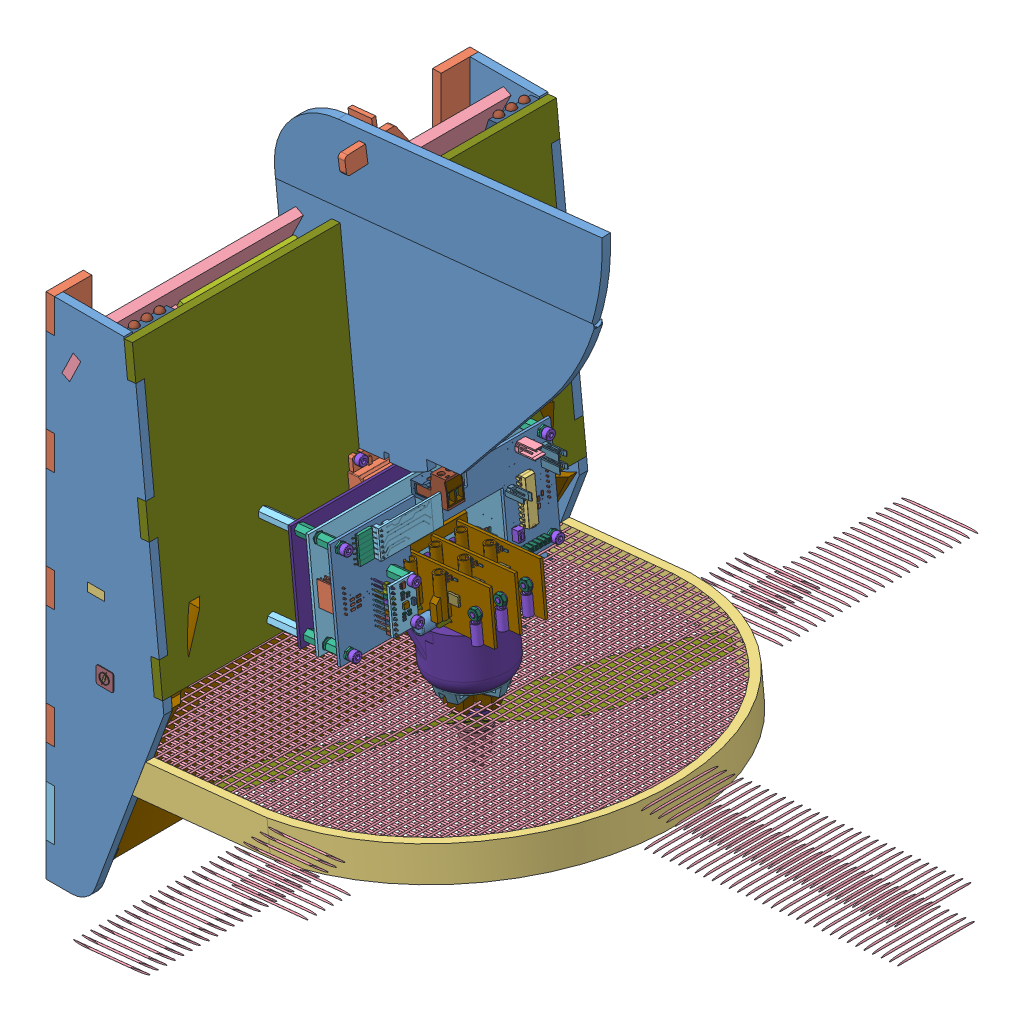
SolidWorks assembly AssTotale, configuration Défaut. Lengths in mm. (continued)
Components (placement in the parent): (continued)
- AssStructSimu-1: AssStructSimu [Défaut] at (-75.9431 -10.8604 24.5323) size (253.25 324.59 251.6) (continued)
  - AssCarte-1: AssCarte [Défaut] at (-42.8534 32.2132 302.028) x (-0.101852 0.9948 0) z (0.9948 0.101852 0) size (67.15 130.57 98.45) (continued)
    - carte_onduleur_v4-1: carte_onduleur_v4 [Défaut] at (-25.7639 0.8332 112.9379) size (66.52 130.57 82.34) (continued)
      - CARTE_ALIM-1: CARTE_ALIM [Défaut] at (-6.4 -57.2 0.803) size (60 130 18.35) (continued)
        - Open CASCADE STEP translator 6.8 1.63.1-1: Open CASCADE STEP translator 6.8 1.63.1 [Défaut] at origin size (60 130 18.35) (continued)
          - Body_1_6-1: Body_1_6 [Défaut] at (7 56 -12) size (60 130 18.35) (continued)
            - 109-1: 109 [Défaut] at (25.4933 -41.1272 0.803) x (-1 0 0) z (0 0 1) size (2.34 1.04 0.5) (continued)
              - =_[0_1_1_45]-1: =_[0_1_1_45] [Défaut] at origin size (2.34 1.04 0.5) (continued)
                - 51-1: 51 [Défaut] at origin size (0.51 1.02 0.5)
            - 111-1: 111 [Défaut] at (22.0269 -41.8272 0.803) x (-1 0 0) z (0 0 1) size (2.34 1.04 0.5)
              - =_[0_1_1_45]-1: =_[0_1_1_45] [Défaut] at origin size (2.34 1.04 0.5)
                - 49_3-1: 49_3 [Défaut] at origin size (2.29 1.04 0.43)
                - 50-1: 50 [Défaut] at (0.3048 0 0) x (-1 0 0) z (0 0 1) size (0.51 1.02 0.5)
                - 51-1: 51 [Défaut] at origin size (0.51 1.02 0.5)
            - 113-1: 113 [Défaut] at (-24.8 -36.7036 0.803) x (0 1 0) z (0 0 1) size (2.34 1.04 0.5)
              - =_[0_1_1_45]-1: =_[0_1_1_45] [Défaut] at origin size (2.34 1.04 0.5)
                - 49_3-1: 49_3 [Défaut] at origin size (2.29 1.04 0.43)
                - 50-1: 50 [Défaut] at (0.3048 0 0) x (-1 0 0) z (0 0 1) size (0.51 1.02 0.5)
                - 51-1: 51 [Défaut] at origin size (0.51 1.02 0.5)
            - 115-1: 115 [Défaut] at (-24.8 -40.3036 0.803) x (0 1 0) z (0 0 1) size (2.34 1.04 0.5)
              - =_[0_1_1_45]-1: =_[0_1_1_45] [Défaut] at origin size (2.34 1.04 0.5)
                - 49_3-1: 49_3 [Défaut] at origin size (2.29 1.04 0.43)
                - 50-1: 50 [Défaut] at (0.3048 0 0) x (-1 0 0) z (0 0 1) size (0.51 1.02 0.5)
                - 51-1: 51 [Défaut] at origin size (0.51 1.02 0.5)
            - 117-1: 117 [Défaut] at (-16 -48.27 0.803) x (0 -1 0) z (0 0 1) size (2.34 1.04 0.5)
              - =_[0_1_1_45]-1: =_[0_1_1_45] [Défaut] at origin size (2.34 1.04 0.5)
                - 49_3-1: 49_3 [Défaut] at origin size (2.29 1.04 0.43)
                - 50-1: 50 [Défaut] at (0.3048 0 0) x (-1 0 0) z (0 0 1) size (0.51 1.02 0.5)
                - 51-1: 51 [Défaut] at origin size (0.51 1.02 0.5)
            - 119-1: 119 [Défaut] at (-22.5189 -47.87 0.803) x (-1 0 0) z (0 0 1) size (2.34 1.04 0.5)
              - =_[0_1_1_45]-1: =_[0_1_1_45] [Défaut] at origin size (2.34 1.04 0.5)
                - 49_3-1: 49_3 [Défaut] at origin size (2.29 1.04 0.43)
                - 50-1: 50 [Défaut] at (0.3048 0 0) x (-1 0 0) z (0 0 1) size (0.51 1.02 0.5)
                - 51-1: 51 [Défaut] at origin size (0.51 1.02 0.5)
            - 121-1: 121 [Défaut] at (22.3933 -38.9272 0.803) size (2.34 1.04 0.5)
              - =_[0_1_1_45]-1: =_[0_1_1_45] [Défaut] at origin size (2.34 1.04 0.5)
                - 49_3-1: 49_3 [Défaut] at origin size (2.29 1.04 0.43)
                - 50-1: 50 [Défaut] at (0.3048 0 0) x (-1 0 0) z (0 0 1) size (0.51 1.02 0.5)
                - 51-1: 51 [Défaut] at origin size (0.51 1.02 0.5)
            - 123-1: 123 [Défaut] at (22.0933 -36.4272 0.803) x (-1 0 0) z (0 0 1) size (2.34 1.04 0.5)
              - =_[0_1_1_45]-1: =_[0_1_1_45] [Défaut] at origin size (2.34 1.04 0.5)
                - 49_3-1: 49_3 [Défaut] at origin size (2.29 1.04 0.43)
                - 50-1: 50 [Défaut] at (0.3048 0 0) x (-1 0 0) z (0 0 1) size (0.51 1.02 0.5)
                - 51-1: 51 [Défaut] at origin size (0.51 1.02 0.5)
            - 125-1: 125 [Défaut] at (22.3933 -32.0272 0.803) x (0 -1 0) z (0 0 1) size (2.34 1.04 0.5)
              - =_[0_1_1_45]-1: =_[0_1_1_45] [Défaut] at origin size (2.34 1.04 0.5)
                - 49_3-1: 49_3 [Défaut] at origin size (2.29 1.04 0.43)
                - 50-1: 50 [Défaut] at (0.3048 0 0) x (-1 0 0) z (0 0 1) size (0.51 1.02 0.5)
                - 51-1: 51 [Défaut] at origin size (0.51 1.02 0.5)
            - 127-1: 127 [Défaut] at (17.9597 -23.1272 0.803) size (2.34 1.04 0.5)
              - =_[0_1_1_16]-1: =_[0_1_1_16] [Défaut] at origin size (2.34 1.04 0.5)
                - 14_2-1: 14_2 [Défaut] at origin size (2.29 1.04 0.43)
                - 15_2-1: 15_2 [Défaut] at (0.3048 0 0) x (-1 0 0) z (0 0 1) size (0.51 1.02 0.5)
                - 16_2-1: 16_2 [Défaut] at origin size (0.51 1.02 0.5)
            - 129-1: 129 [Défaut] at (20.0269 -24.9272 0.803) x (-1 0 0) z (0 0 1) size (2.34 1.04 0.5)
              - =_[0_1_1_16]-1: =_[0_1_1_16] [Défaut] at origin size (2.34 1.04 0.5)
                - 14_2-1: 14_2 [Défaut] at origin size (2.29 1.04 0.43)
                - 15_2-1: 15_2 [Défaut] at (0.3048 0 0) x (-1 0 0) z (0 0 1) size (0.51 1.02 0.5)
                - 16_2-1: 16_2 [Défaut] at origin size (0.51 1.02 0.5)
            - 131-1: 131 [Défaut] at (16.9933 -37.5272 0.803) x (-1 0 0) z (0 0 1) size (2.34 1.04 0.5)
              - =_[0_1_1_45]-1: =_[0_1_1_45] [Défaut] at origin size (2.34 1.04 0.5)
                - 49_3-1: 49_3 [Défaut] at origin size (2.29 1.04 0.43)
                - 50-1: 50 [Défaut] at (0.3048 0 0) x (-1 0 0) z (0 0 1) size (0.51 1.02 0.5)
                - 51-1: 51 [Défaut] at origin size (0.51 1.02 0.5)
            - 136-1: 136 [Défaut] at (3.2957 -29.23 0.803) x (-1 0 0) z (0 0 1) size (4.78 2.79 2.03)
              - =_[0_1_1_110]_2-1: =_[0_1_1_110]_2 [Défaut] at origin size (4.78 2.79 2.03)
                - 132-1: 132 [Défaut] at origin size (4.32 2.79 1.78)
                - 133-1: 133 [Défaut] at (0.4572 0 0) x (-1 0 0) z (0 0 1) size (1.02 1.27 1.32)
                - 134-1: 134 [Défaut] at origin size (1.02 1.27 1.32)
            - 141-1: 141 [Défaut] at (0.2436 -33.3673 0.803) size (3.35 1.3 0.55)
              - =_[0_1_1_115]_2-1: =_[0_1_1_115]_2 [Défaut] at origin size (3.35 1.3 0.55)
                - 137-1: 137 [Défaut] at origin size (3.3 1.3 0.48)
                - 138-1: 138 [Défaut] at (0.5588 0 0) x (-1 0 0) z (0 0 1) size (0.76 1.27 0.55)
                - 139-1: 139 [Défaut] at origin size (0.76 1.27 0.55)
            - 143_2-1: 143_2 [Défaut] at (-0.3 -45.47 0.803) x (0 1 0) z (0 0 1) size (2.34 1.04 0.5)
              - =_[0_1_1_16]-1: =_[0_1_1_16] [Défaut] at origin size (2.34 1.04 0.5)
                - 14_2-1: 14_2 [Défaut] at origin size (2.29 1.04 0.43)
                - 15_2-1: 15_2 [Défaut] at (0.3048 0 0) x (-1 0 0) z (0 0 1) size (0.51 1.02 0.5)
                - 16_2-1: 16_2 [Défaut] at origin size (0.51 1.02 0.5)
            - 145-1: 145 [Défaut] at (6.6 31.13 0.803) x (0 1 0) z (0 0 1) size (3.35 1.3 0.55)
              - =_[0_1_1_25]_2-1: =_[0_1_1_25]_2 [Défaut] at origin size (3.35 1.3 0.55)
                - 24-1: 24 [Défaut] at origin size (3.3 1.3 0.48)
                - 25_2-1: 25_2 [Défaut] at (0.5588 0 0) x (-1 0 0) z (0 0 1) size (0.76 1.27 0.55)
                - 26_2-1: 26_2 [Défaut] at origin size (0.76 1.27 0.55)
            - 148-1: 148 [Défaut] at (-7.5 -56.57 0.803) size (15.24 2.54 7.37)
              - =_[0_1_1_122]_2-1: =_[0_1_1_122]_2 [Défaut] at origin size (15.24 2.54 7.37)
                - 146-1: 146 [Défaut] at (6.3 0 1) x (1 0 0) z (0 -1 0) size (15.24 7.37 2.54)
            - 150-1: 150 [Défaut] at (-26.3 -45.9 0.803) x (0 1 0) z (0 0 1) size (2.34 1.04 0.5)
              - =_[0_1_1_45]-1: =_[0_1_1_45] [Défaut] at origin size (2.34 1.04 0.5)
                - 49_3-1: 49_3 [Défaut] at origin size (2.29 1.04 0.43)
                - 50-1: 50 [Défaut] at (0.3048 0 0) x (-1 0 0) z (0 0 1) size (0.51 1.02 0.5)
                - 51-1: 51 [Défaut] at origin size (0.51 1.02 0.5)
    - AssEntretoise-1: AssEntretoise [Défaut] at (-50.7639 -62.5535 129.2811) x (0 0 -1) z (1 0 0) size (58.24 7.29 7.81)
      - socket head cap screw 4762_din-1: socket head cap screw 4762_din [EN ISO 4762 M3 x 5 - 5N] at (-2.4967 0.5867 0) size (8 5.5 5.5)
      - hexagonal_spacer_MF_M3_H20_HEX5.5_FTD6_MTL6-1: hexagonal_spacer_MF_M3_H20_HEX5.5_FTD6_MTL6 [Défaut] at (48.3433 0.5867 0) x (0 0 1) z (-1 0 0) size (6.36 5.51 26)
      - hex nut style 1 gradeab_din-1: hex nut style 1 gradeab_din [Hexagon Nut ISO 4032 - M3 - W - N] at (53.3433 0.5867 0) x (0 0.943962 0.330053) z (-1 0 0) size (5.5 6.35 2.4)
      - hexagonal_spacer_MF_M3_H12_HEX5.5_FTD6_MTL6-2: hexagonal_spacer_MF_M3_H12_HEX5.5_FTD6_MTL6 [Défaut] at (27.0633 0.5867 0) x (0 0.248308 0.968681) z (-1 0 0) size (6.36 5.51 18)
      - hexagonal_spacer_MF_M3_H12_HEX5.5_FTD6_MTL6-3: hexagonal_spacer_MF_M3_H12_HEX5.5_FTD6_MTL6 [Défaut] at (13.7833 0.5867 0) x (0 0 1) z (-1 0 0) size (6.36 5.51 18)
    - AssEntretoise-2: AssEntretoise [Défaut] at (0.4521 -62.0374 129.2811) x (0 0 -1) z (0.694658 0.71934 0) size (58.24 7.29 7.81)
      - socket head cap screw 4762_din-1: socket head cap screw 4762_din [EN ISO 4762 M3 x 5 - 5N] at (-2.4967 0.5867 0) size (8 5.5 5.5)
      - hexagonal_spacer_MF_M3_H20_HEX5.5_FTD6_MTL6-1: hexagonal_spacer_MF_M3_H20_HEX5.5_FTD6_MTL6 [Défaut] at (48.3433 0.5867 0) x (0 0 1) z (-1 0 0) size (6.36 5.51 26)
      - hex nut style 1 gradeab_din-1: hex nut style 1 gradeab_din [Hexagon Nut ISO 4032 - M3 - W - N] at (53.3433 0.5867 0) x (0 0.943962 0.330053) z (-1 0 0) size (5.5 6.35 2.4)
      - hexagonal_spacer_MF_M3_H12_HEX5.5_FTD6_MTL6-2: hexagonal_spacer_MF_M3_H12_HEX5.5_FTD6_MTL6 [Défaut] at (27.0633 0.5867 0) x (0 0.248308 0.968681) z (-1 0 0) size (6.36 5.51 18)
      - hexagonal_spacer_MF_M3_H12_HEX5.5_FTD6_MTL6-3: hexagonal_spacer_MF_M3_H12_HEX5.5_FTD6_MTL6 [Défaut] at (13.7833 0.5867 0) x (0 0 1) z (-1 0 0) size (6.36 5.51 18)
    - AssEntretoise-3: AssEntretoise [Défaut] at (-51.9799 58.1038 129.2811) x (0 0 -1) z (-0.694658 -0.71934 0) size (58.24 7.29 7.81)
      - socket head cap screw 4762_din-1: socket head cap screw 4762_din [EN ISO 4762 M3 x 5 - 5N] at (-2.4967 0.5867 0) size (8 5.5 5.5)
      - hexagonal_spacer_MF_M3_H20_HEX5.5_FTD6_MTL6-1: hexagonal_spacer_MF_M3_H20_HEX5.5_FTD6_MTL6 [Défaut] at (48.3433 0.5867 0) x (0 0 1) z (-1 0 0) size (6.36 5.51 26)
      - hex nut style 1 gradeab_din-1: hex nut style 1 gradeab_din [Hexagon Nut ISO 4032 - M3 - W - N] at (53.3433 0.5867 0) x (0 0.943962 0.330053) z (-1 0 0) size (5.5 6.35 2.4)
      - hexagonal_spacer_MF_M3_H12_HEX5.5_FTD6_MTL6-2: hexagonal_spacer_MF_M3_H12_HEX5.5_FTD6_MTL6 [Défaut] at (27.0633 0.5867 0) x (0 0.248308 0.968681) z (-1 0 0) size (6.36 5.51 18)
      - hexagonal_spacer_MF_M3_H12_HEX5.5_FTD6_MTL6-3: hexagonal_spacer_MF_M3_H12_HEX5.5_FTD6_MTL6 [Défaut] at (13.7833 0.5867 0) x (0 0 1) z (-1 0 0) size (6.36 5.51 18)
    - AssEntretoise-4: AssEntretoise [Défaut] at (0.2897 58.1744 129.2811) x (0 0 -1) z (-0.999848 0.017452 0) size (58.24 7.29 7.81)
      - socket head cap screw 4762_din-1: socket head cap screw 4762_din [EN ISO 4762 M3 x 5 - 5N] at (-2.4967 0.5867 0) size (8 5.5 5.5)
      - hexagonal_spacer_MF_M3_H20_HEX5.5_FTD6_MTL6-1: hexagonal_spacer_MF_M3_H20_HEX5.5_FTD6_MTL6 [Défaut] at (48.3433 0.5867 0) x (0 0 1) z (-1 0 0) size (6.36 5.51 26)
      - hex nut style 1 gradeab_din-1: hex nut style 1 gradeab_din [Hexagon Nut ISO 4032 - M3 - W - N] at (53.3433 0.5867 0) x (0 0.943962 0.330053) z (-1 0 0) size (5.5 6.35 2.4)
      - hexagonal_spacer_MF_M3_H12_HEX5.5_FTD6_MTL6-2: hexagonal_spacer_MF_M3_H12_HEX5.5_FTD6_MTL6 [Défaut] at (27.0633 0.5867 0) x (0 0.248308 0.968681) z (-1 0 0) size (6.36 5.51 18)
      - hexagonal_spacer_MF_M3_H12_HEX5.5_FTD6_MTL6-3: hexagonal_spacer_MF_M3_H12_HEX5.5_FTD6_MTL6 [Défaut] at (13.7833 0.5867 0) x (0 0 1) z (-1 0 0) size (6.36 5.51 18)
    - AssMpu-1: AssMpu [Défaut] at (-44.7921 29.4106 121.7839) size (8 8 22.28)
      - hex nut style 1 gradeab_din-1: hex nut style 1 gradeab_din [Hexagon Nut ISO 4032 - M3 - W - N] at (0.2783 0.3227 1.2) size (5.5 6.35 2.4)
      - plain washer 6903 type ab_din-1: plain washer 6903 type ab_din [DIN 6903-A3] at (0.2783 0.3227 1.2) x (0 0 1) z (-1 0 0) size (1 8 8)
      - socket head cap screw 4762_din-1: socket head cap screw 4762_din [EN ISO 4762 M3 x 5 - 5N] at (0.2783 0.3227 19.76) x (0 0 -1) z (-0.852155 0.523289 0) size (8 5.5 5.5)
      - hexagonal_spacer_MF_M3_H12_HEX5.5_FTD6_MTL6-1: hexagonal_spacer_MF_M3_H12_HEX5.5_FTD6_MTL6 [Défaut] at (0.2783 0.3227 3.48) size (6.36 5.51 18)
    - AssMpu-2: AssMpu [Défaut] at (-24.7921 29.4106 121.7839) size (8 8 22.28)
      - hex nut style 1 gradeab_din-1: hex nut style 1 gradeab_din [Hexagon Nut ISO 4032 - M3 - W - N] at (0.2783 0.3227 1.2) size (5.5 6.35 2.4)
      - plain washer 6903 type ab_din-1: plain washer 6903 type ab_din [DIN 6903-A3] at (0.2783 0.3227 1.2) x (0 0 1) z (-1 0 0) size (1 8 8)
      - socket head cap screw 4762_din-1: socket head cap screw 4762_din [EN ISO 4762 M3 x 5 - 5N] at (0.2783 0.3227 19.76) x (0 0 -1) z (-0.852155 0.523289 0) size (8 5.5 5.5)
      - hexagonal_spacer_MF_M3_H12_HEX5.5_FTD6_MTL6-1: hexagonal_spacer_MF_M3_H12_HEX5.5_FTD6_MTL6 [Défaut] at (0.2783 0.3227 3.48) size (6.36 5.51 18)
    - AssCosse-1: AssCosse [Défaut] at (-36.6204 16.2367 163.5671) x (0 1 0) z (-0.344896 0 0.938641) size (9.83 18.66 11.64)
      - socket head cap screw 4762_din-1: socket head cap screw 4762_din [EN ISO 4762 M3 x 6 - 6N] at (-5.1064 0.3659 0) size (9 5.5 5.5)
      - plain washer 6903 type ab_din-1: plain washer 6903 type ab_din [DIN 6903-A3] at (-2.1064 0.3659 0) size (1 8 8)
      - hex nut style 1 gradeab_din-2: hex nut style 1 gradeab_din [Hexagon Nut ISO 4032 - M3 - W - N] at (1.281 0.3659 0) x (0 0.924225 0.381849) z (-1 0 0) size (5.5 6.35 2.4)
      - 31880-1: 31880 [Default] at (0.4936 0.3659 0) x (0 0.344896 -0.938641) z (0 -0.938641 -0.344896) size (5.54 5 17.37)
    - AssCosse-2: AssCosse [Défaut] at (-36.6204 1.2367 163.5671) x (0 1 0) z (-0.344896 0 0.938641) size (9.83 18.66 11.64)
      - socket head cap screw 4762_din-1: socket head cap screw 4762_din [EN ISO 4762 M3 x 6 - 6N] at (-5.1064 0.3659 0) size (9 5.5 5.5)
      - plain washer 6903 type ab_din-1: plain washer 6903 type ab_din [DIN 6903-A3] at (-2.1064 0.3659 0) size (1 8 8)
      - hex nut style 1 gradeab_din-2: hex nut style 1 gradeab_din [Hexagon Nut ISO 4032 - M3 - W - N] at (1.281 0.3659 0) x (0 0.924225 0.381849) z (-1 0 0) size (5.5 6.35 2.4)
      - 31880-1: 31880 [Default] at (0.4936 0.3659 0) x (0 0.344896 -0.938641) z (0 -0.938641 -0.344896) size (5.54 5 17.37)
    - AssCosse-3: AssCosse [Défaut] at (-36.6204 -13.7633 163.5671) x (0 1 0) z (-0.344896 0 0.938641) size (9.83 18.66 11.64)
      - socket head cap screw 4762_din-1: socket head cap screw 4762_din [EN ISO 4762 M3 x 6 - 6N] at (-5.1064 0.3659 0) size (9 5.5 5.5)
      - plain washer 6903 type ab_din-1: plain washer 6903 type ab_din [DIN 6903-A3] at (-2.1064 0.3659 0) size (1 8 8)
      - hex nut style 1 gradeab_din-2: hex nut style 1 gradeab_din [Hexagon Nut ISO 4032 - M3 - W - N] at (1.281 0.3659 0) x (0 0.924225 0.381849) z (-1 0 0) size (5.5 6.35 2.4)
      - 31880-1: 31880 [Default] at (0.4936 0.3659 0) x (0 0.344896 -0.938641) z (0 -0.938641 -0.344896) size (5.54 5 17.37)
    - Terminal_QD_Female-1: Terminal_QD_Female [Default] at (-33.4139 20.2862 128.1409) x (0 1 0) z (-1 0 0) size (9.4 5.5 22.35)
    - Terminal_QD_Female-2: Terminal_QD_Female [Default] at (-33.4139 5.2862 128.1409) x (0 1 0) z (-1 0 0) size (9.4 5.5 22.35)
    - Terminal_QD_Female-3: Terminal_QD_Female [Default] at (-33.4139 -9.7138 128.1409) x (0 1 0) z (-1 0 0) size (9.4 5.5 22.35)
    - Terminal_QD_Female-4: Terminal_QD_Female [Default] at (-33.4139 -9.7138 145.1409) x (0 1 0) z (-1 0 0) size (9.4 5.5 22.35)
    - Terminal_QD_Female-5: Terminal_QD_Female [Default] at (-33.4139 5.2862 145.1409) x (0 1 0) z (-1 0 0) size (9.4 5.5 22.35)
    - Terminal_QD_Female-6: Terminal_QD_Female [Default] at (-33.4139 20.2862 145.1409) x (0 1 0) z (-1 0 0) size (9.4 5.5 22.35)
- Parallax-Servo-Horn-1: Parallax-Servo-Horn [Défaut] at (-19.4936 17.1266 324.6266) x (0.097568 -0.952956 0.286975) z (0.9948 0.101852 0) size (38.81 38.81 6.17)
- NTM_35-36_engine_assembly-1: NTM_35-36_engine_assembly [Défaut] at (21.4411 -39.9993 324.5222) x (-0.837214 -0.085718 -0.540116) z (-0.537307 -0.055012 0.841591) size (60.56 77.2 246.41)
  - engine_base-1: engine_base [Défaut] at (-1.8719 -19.5526 -1.1165) x (0 1 0) z (0 0 1) size (6.8 35 35)
  - engine_bearing-1: engine_bearing [Défaut] at origin size (10 4 10)
  - Propeller_cone-1: Propeller_cone [Défaut] at (-1.8719 33.6474 -4.1165) x (1 0 0) z (0 1 0) size (17.6 17.6 24)
  - engine_bearing-2: engine_bearing [Défaut] at (0 22.8 0) size (10 4 10)
  - NTM_35-36_enginebody-1: NTM_35-36_enginebody [Défaut] at (-1.8719 -12.7526 -1.1165) size (35 31.7 35)
  - Stator-1: Stator [Défaut] at origin size (27.75 22.36 27.94)
  - propellers_10x4-1: propellers_10x4 [Défaut] at (-6.8719 27.4474 -4.9165) size (60.56 10.53 246.41)
  - propeller_washer-1: propeller_washer [Défaut] at (-1.8719 24.4474 -1.1165) x (0 1 0) z (0 0 1) size (2.5 18 18)
  - Propeller_adaptor-1: Propeller_adaptor [Défaut] at (2.1948 17.1101 -3.713) size (23.46 32.5 25)
- AssGouv-1: AssGouv [Défaut] at (16.5802 187.593 125.4395) x (0.9948 0.101852 0) z (0.004047 -0.039527 0.99921) size (200.18 52.5 43.47)
  - P10_1-1: P10_1 [Défaut] at (-108.1667 -19.4144 197.6829) size (200.18 50.13 5)
  - attache_pale-1: attache_pale [Défaut] at (-49.1667 8.0856 190.1829) x (0 0 -1) z (-1 0 0) size (43.47 35 14)
- AssTige-1: AssTige [Défaut] at (129.5074 132.411 306.7114) x (-0.101734 0.99365 -0.048063) z (-0.9948 -0.101852 0) size (166.39 7.19 19)
  - tige_servo-1: tige_servo [Défaut] at (-106.2712 0.2685 162) size (165 6 6)
  - socket head cap screw 4762_din-2: socket head cap screw 4762_din [EN ISO 4762 M2 x 10 - 10N] at (-104.2712 3.2685 170) x (0 0 -1) z (0.923728 0.383049 0) size (12 3.8 3.8)
  - hex nut style 1 gradeab_din-1: hex nut style 1 gradeab_din [Hexagon Nut ISO 4032 - M3 - W - N] at (55.7288 3.2685 156) size (5.5 6.35 2.4)
  - hex nut style 1 gradeab_din-2: hex nut style 1 gradeab_din [Hexagon Nut ISO 4032 - M2 - W - N] at (-104.2712 3.2685 160) x (0.904801 0.425836 0) z (0 0 1) size (4 4.62 1.6)
  - socket head cap screw 4762_din-3: socket head cap screw 4762_din [EN ISO 4762 M3 x 16 - 16N] at (55.7288 3.2685 171) x (0 0 -1) z (0.923728 0.383049 0) size (19 5.5 5.5)
- AssGoPro-1: AssGoPro [Défaut] at (-71.2437 -28.2623 330.8954) x (0 0 1) z (-0.103167 0.994664 0) size (64.3 52.3 34.42)
  - GoPRo Frame for LCD Screen-1: GoPRo Frame for LCD Screen [Défaut] at (-2.6935 10.9558 5.5635) size (64.3 59.3 34.42)
    - GoProFrame MJM-1: GoProFrame MJM [Défaut] at (-3.6084 -1.6692 52.45) size (64.3 47.42 23.68)
    - GoPro Hero 3 Front Panel-1: GoPro Hero 3 Front Panel [Défaut] at (-3.6084 -1.6692 55.7) x (-1 0 0) z (0 0 -1) size (59.25 41.2 1.9)
    - GoPro Hero 3 Screen-1: GoPro Hero 3 Screen [Défaut] at (12.7166 3.9308 54.9) size (15 18 1)
    - GoPro Hero 3 Mode Button-1: GoPro Hero 3 Mode Button [Défaut] at (13.4166 -12.4692 54.95) x (-1 0 0) z (0 0 -1) size (11.97 12.11 3.03)
    - GoPro Hero 3 LED Cover-1: GoPro Hero 3 LED Cover [Défaut] at (3.1166 -9.3192 54.85) x (-0.999988 0.004848 0) z (0 0 -1) size (5 5 1.4)
    - GoPro Hero 3 LED Cover-2: GoPro Hero 3 LED Cover [Défaut] at (3.1166 -16.0692 54.85) x (-0.999988 0.004848 0) z (0 0 -1) size (5 5 1.4)
    - GoPro Hero 3 Housing-1: GoPro Hero 3 Housing [Défaut] at (-3.6084 -1.6692 55.7) size (59.37 41.3 29.84)
    - GoPro Hero 3 Lens-1: GoPro Hero 3 Lens [Défaut] at (-18.9334 5.6308 47.35) x (-0.380542 -0.924764 0) z (0 0 -1) size (13.71 15.7 7.94)
    - GoPro Hero 3 Indicator Cover-1: GoPro Hero 3 Indicator Cover [Défaut] at (-25.5834 -22.2692 69.9) x (-0.997412 0 -0.0719) z (0 1 0) size (3 3 2)
    - GoPro Hero 3 Indicator Cover-2: GoPro Hero 3 Indicator Cover [Défaut] at (-28.8834 12.2308 73) x (-0.999992 0.004018 0) z (0 0 1) size (3 3 2)
    - GoPro Hero 3 Indicator Cover-3: GoPro Hero 3 Indicator Cover [Défaut] at (20.6666 16.9308 58.4) x (-0.997739 0 -0.067212) z (0 1 0) size (3 3 2)
    - slot-1: slot [Défaut] at (-24.7434 -9.7363 65.05) x (0 1 0) z (0 0 -1) size (16 15.02 2.44)
    - GoPro Hero 3 HDMI pin-1: GoPro Hero 3 HDMI pin [Défaut] at (-26.982 2.9815 24.7172) x (0.105491 0.98175 -0.158237) z (-0.992872 0.095109 -0.071829) size (3.29 0.86 3.28)
  - support1-2: support1 [Défaut] at (-1.3019 -18.8633 67.0135) x (0 0 1) z (-1 0 0) size (5 5 10)
Mates (geometry in assembly coordinates):
- Coaxiale6: concentric aligned: cylinder of AssStructSimu-1/AssToitMot-1/Parallax-Servo_DUMMY-1 through (-20.8328 16.9895 324.6266) axis (-0.9948 -0.101852 0) radius 2.9845; cylinder of Parallax-Servo-Horn-1 through (-20.8328 16.9895 324.6266) axis (-0.9948 -0.101852 0) radius 2.9845
- Coïncidente9: coincident anti-aligned: plane of AssStructSimu-1/AssToitMot-1/Parallax-Servo_DUMMY-1 through (-25.002 16.5626 324.6266) normal (0.9948 0.101852 0); plane of Parallax-Servo-Horn-1 through (-25.002 16.5626 324.6266) normal (-0.9948 -0.101852 0)
- Coaxiale9: concentric aligned: cylinder of AssStructSimu-1/AssToitMot-1/AssToit-1/P12-1 through (22.126 -25.3005 324.5936) axis (-0.101852 0.9948 0) radius 17.5; cylinder of NTM_35-36_engine_assembly-1/NTM_35-36_enginebody-1 through (24.601 -49.4741 324.5936) axis (-0.101852 0.9948 0) radius 17.5
- Coïncidente11: coincident aligned: plane of AssStructSimu-1/AssToitMot-1/AssToit-1/P12-1 through (21.6167 -20.3265 324.5936) normal (-0.101852 0.9948 0); plane of NTM_35-36_engine_assembly-1/engine_base-1 through (36.2679 -18.8264 334.0456) normal (-0.101852 0.9948 0)
- Coaxiale10: concentric anti-aligned: cylinder of AssStructSimu-1/AssToitMot-1/AssToit-1/P10_2-1 through (99.5361 166.0791 324.5936) axis (-0.9948 -0.101852 0) radius 2.5; cylinder of AssGouv-1/P10_1-1 through (-87.9836 146.8801 324.5936) axis (0.9948 0.101852 0) radius 2.5
- Tangent1: tangent anti-aligned: cylinder of AssGouv-1/P10_1-1 through (-45.5263 214.0752 329.5817) axis (-0.004047 0.039527 -0.99921) radius 151.8495; circle of AssStructSimu-1/AssToitMot-1/AssToit-1/P10_2-1
- Coaxiale11: concentric anti-aligned: cylinder of AssGouv-1/attache_pale-1 through (-34.4587 164.0964 296.4709) axis (0.9948 0.101852 0) radius 1.5; cylinder of ? through (-77.0996 159.7306 296.4709) axis (-0.9948 -0.101852 0) radius 1.5
- Coaxiale12: concentric aligned: cylinder of Parallax-Servo-Horn-1 through (-19.0048 12.3526 308.4582) axis (-0.9948 -0.101852 0) radius 0.635; cylinder of AssTige-1/socket head cap screw 4762_din-2 through (-60.5695 8.0971 308.4582) axis (-0.9948 -0.101852 0) radius 1
- Coïncidente12: coincident anti-aligned: plane of Parallax-Servo-Horn-1 through (-20.7141 9.0976 320.3887) normal (-0.9948 -0.101852 0); plane of AssTige-1/tige_servo-1 through (-20.8374 10.3018 311.5508) normal (0.9948 0.101852 0)
- Coaxiale13: concentric anti-aligned: cylinder of AssGouv-1/attache_pale-1 through (-35.2009 171.3449 300.7682) axis (0.9948 0.101852 0) radius 1.5; cylinder of AssTige-1/socket head cap screw 4762_din-3 through (-77.8418 166.9792 300.7682) axis (-0.9948 -0.101852 0) radius 1.5
- Coaxiale14: concentric anti-aligned: cylinder of AssStructSimu-1/AssBase-1/support2-1 through (-94.6912 39.1921 314.5936) axis (0 0 1) radius 1.5; cylinder of AssGoPro-1/support1-2 through (-94.6912 39.1921 329.5936) axis (0 0 -1) radius 1.5
- Coïncidente13: coincident anti-aligned: plane of AssStructSimu-1/AssBase-1/support2-1 through (-92.1479 41.6481 329.5936) normal (0 0 -1); plane of AssGoPro-1/support1-2 through (-96.9199 36.4475 329.5936) normal (0 0 1)
